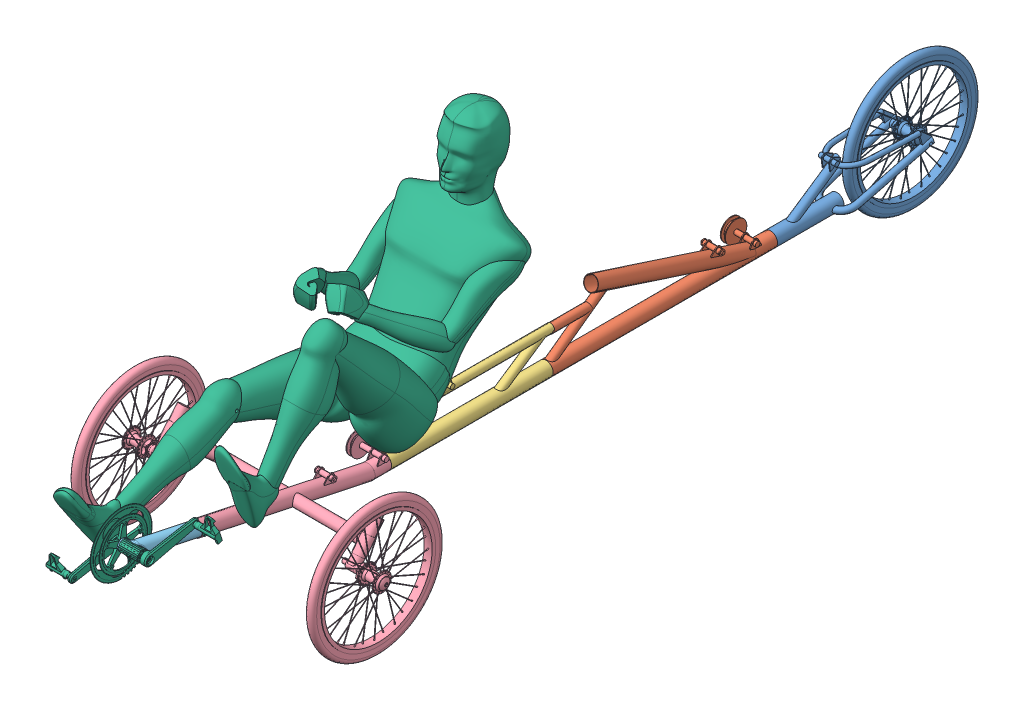
SolidWorks assembly Assem, configuration Default. Lengths in mm.
Overall size (938 1194.09 3282.57).
6 component instances, 6 part files, 14 mates.
Components (placement in the parent):
- Part1-1: Part1 [Default] at (162.4265 593.6834 583.9361) size (187.74 478.75 741.31)
- Part4-1: Part4 [Default] at (162.4265 593.6834 1394.9361) x (-1 0 0) z (0 0 -1) size (108.38 235.55 819.31)
- Part2-1: Part2 [Default] at (162.4265 593.6834 1418.4461) x (-1 0 0) z (0 0 -1) size (66 183.4 600)
- Front-1: Front [Default] at (162.4265 725.2294 2660.5124) x (-1 0 0) z (0 -0.207912 -0.978148) size (938 478.75 717.85)
- buis_voor_trappers-1: buis_voor_trappers [Default] at (162.4265 774.3001 2891.3723) x (1 0 0) z (0 0.207912 0.978148) size (73.98 47.1 420)
- man and pedals-2: man and pedals [Default] at (536.9701 201.7009 2682.2799) x (0 0.086963 -0.996212) z (1 0 0) size (1598.05 832.63 470.97)
Mates (geometry in assembly coordinates):
- Coincident1: coincident anti-aligned: circle of Part1-1; circle of Part4-1
- Parallel2: parallel aligned: plane of Part4-1 through (112.1265 627.5678 657.7361) normal (1 0 0); plane of assembly through (0 0 0) normal (1 0 0)
- Concentric2: concentric aligned: circle of Part4-1; circle of Part2-1
- Coincident3: coincident anti-aligned: plane of Part4-1 through (162.4265 593.6834 1394.9361) normal (0 0 1); plane of Part2-1 through (162.4265 593.6834 1394.9361) normal (0 0 -1)
- Parallel4: parallel anti-aligned: plane of Part2-1 through (128.0265 737.3334 1764.4719) normal (-1 0 0); plane of assembly through (0 0 0) normal (1 0 0)
- Concentric3: concentric anti-aligned: circle of Front-1; circle of Part2-1
- Coincident4: coincident anti-aligned: plane of Part2-1 through (162.4265 593.6834 1978.9361) normal (0 0 1); plane of Front-1 through (162.4265 593.6834 1978.9361) normal (0 0 -1)
- Parallel5: parallel anti-aligned: plane of Front-1 through (84.6265 627.5671 2001.6569) normal (-1 0 0); plane of assembly through (0 0 0) normal (1 0 0)
- Concentric4: concentric aligned: cylinder of Front-1 through (162.4265 600.4824 2073.6239) axis (0 0.207912 0.978148) radius 24.2; cylinder of buis_voor_trappers-1 through (162.4265 691.1355 2500.1132) axis (0 0.207912 0.978148) radius 23.55
- Tangent1: tangent aligned: plane of Part4-1 through (93.6265 632.0158 657.7361) normal (-1 0 0); face of ?
- Concentric5: concentric aligned: cylinder of buis_voor_trappers-1 through (200.8265 790.6656 2968.3656) axis (-1 0 0) radius 17.15; circle of ?
- Parallel6: parallel aligned: plane of buis_voor_trappers-1 through (200.8265 774.3001 2891.3723) normal (1 0 0); plane of assembly through (0 0 0) normal (1 0 0)
- Concentric6: concentric anti-aligned: cylinder of buis_voor_trappers-1 through (200.8265 774.3001 2891.3723) axis (-1 0 0) radius 17.15; cylinder of man and pedals-2 through (196.209 774.3001 2891.3723) axis (1 0 0) radius 20
- Coincident9: coincident anti-aligned: circle of buis_voor_trappers-1; circle of man and pedals-2
